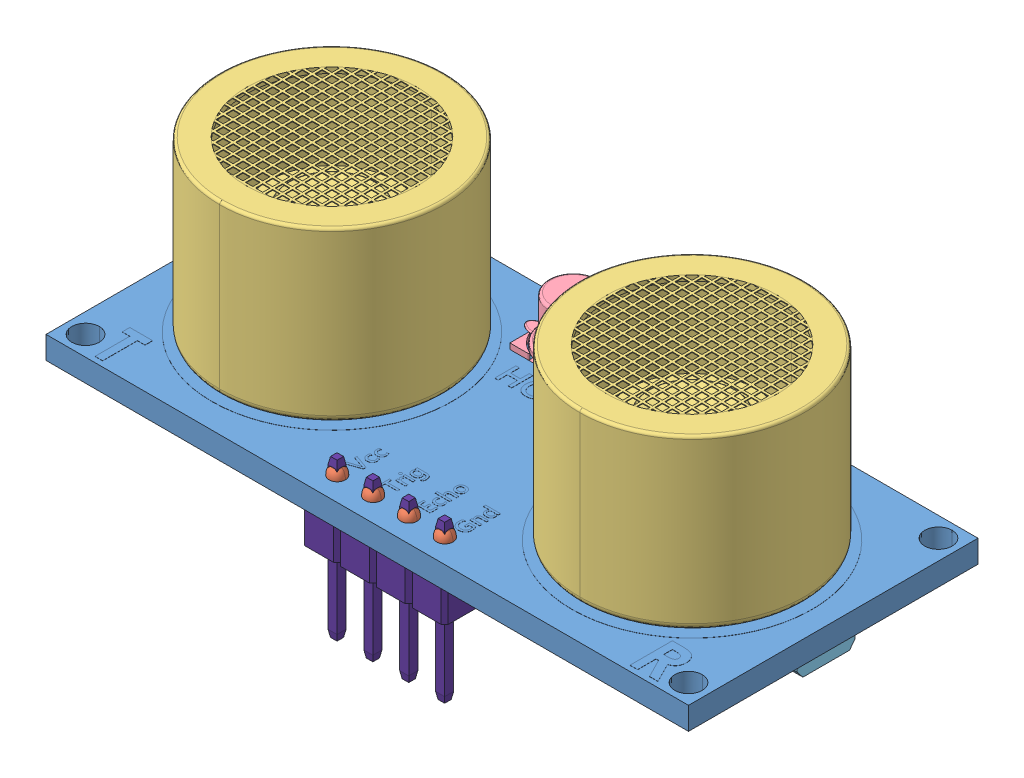
SolidWorks assembly mc_HC-SR04, configuration По умолчанию. Lengths in mm.
Overall size (45.5 21.95 20.5).
46 component instances, 17 part files, 0 mates.
Components (placement in the parent):
- HC-SR04.STEP-1: HC-SR04.STEP [Default] at origin size (45.5 21.95 20.5)
  - HC-SR04board.STEP-1: HC-SR04board.STEP [Default] at origin size (45.5 1.61 20.5)
  - solder.STEP-1: solder.STEP [Default] at (-3.8014 1.6 8.5727) size (1.17 0.65 1.17)
  - solder.STEP-2: solder.STEP [Default] at (-1.2614 1.6 8.5727) size (1.17 0.65 1.17)
  - solder.STEP-3: solder.STEP [Default] at (1.2786 1.6 8.5727) size (1.17 0.65 1.17)
  - solder.STEP-4: solder.STEP [Default] at (3.8186 1.6 8.5727) size (1.17 0.65 1.17)
  - Emitter.STEP-1: Emitter.STEP [Default] at (-12.75 1.6 0) size (15.9 15.2 15.9)
  - Emitter.STEP-2: Emitter.STEP [Default] at (12.75 1.6 0) size (15.9 15.2 15.9)
  - CrystalOscillator.STEP-1: CrystalOscillator.STEP [Default] at (0 1.6 -7.5) size (13.3 6.4 4.5)
  - solder.STEP-5: solder.STEP [Default] at (-2.0167 0 -7.5286) x (-0.837169 0 -0.546944) z (-0.546944 0 0.837169) size (1.17 0.65 1.17)
  - solder.STEP-6: solder.STEP [Default] at (1.9833 0 -7.5286) x (-0.837169 0 -0.546944) z (-0.546944 0 0.837169) size (1.17 0.65 1.17)
  - smdChip14pin.STEP-1: smdChip14pin.STEP [Default] at (22.25 -0.725 0) x (0 0 -1) z (-1 0 0) size (7.3 1.22 8.75)
  - smdChip14pin.STEP-2: smdChip14pin.STEP [Default] at (4.375 -0.725 0) x (0 0 -1) z (-1 0 0) size (7.3 1.22 8.75)
  - smdChip16pin.STEP-1: smdChip16pin.STEP [Default] at (-18.6 -0.725 5) x (1 0 0) z (0 0 -1) size (7.3 1.22 10)
  - smdceramiccapacitor.STEP-1: smdceramiccapacitor.STEP [Default] at (17.8499 0 -5.5522) x (0 0 -1) z (-1 0 0) size (2.52 0.61 1.3)
  - smdceramiccapacitor.STEP-2: smdceramiccapacitor.STEP [Default] at (17.8499 0 5.585) x (0 0 -1) z (-1 0 0) size (2.52 0.61 1.3)
  - smdceramiccapacitor.STEP-3: smdceramiccapacitor.STEP [Default] at (15.2359 0 8.7006) x (-1 0 0) z (0 0 1) size (2.52 0.61 1.3)
  - smdceramiccapacitor.STEP-4: smdceramiccapacitor.STEP [Default] at (8.3844 0 0.0383) x (-1 0 0) z (0 0 1) size (2.52 0.61 1.3)
  - smdceramiccapacitor.STEP-5: smdceramiccapacitor.STEP [Default] at (8.3844 0 -4.7577) x (-1 0 0) z (0 0 1) size (2.52 0.61 1.3)
  - smdceramiccapacitor.STEP-6: smdceramiccapacitor.STEP [Default] at (8.3844 0 -2.3108) x (-1 0 0) z (0 0 1) size (2.52 0.61 1.3)
  - smdceramiccapacitor.STEP-7: smdceramiccapacitor.STEP [Default] at (-7.8145 0 -2.3108) x (-1 0 0) z (0 0 1) size (2.52 0.61 1.3)
  - smdResistor753.STEP-1: smdResistor753.STEP [Default] at (20.6199 0 5.0565) x (-1 0 0) z (0 0 1) size (2.53 0.63 1.31)
  - smdResistor753.STEP-2: smdResistor753.STEP [Default] at (-7.7732 0 -0.1429) x (-1 0 0) z (0 0 1) size (2.53 0.63 1.31)
  - smdResistor753.STEP-3: smdResistor753.STEP [Default] at (20.6199 0 -4.936) x (-1 0 0) z (0 0 1) size (2.53 0.63 1.31)
  - smdResistor392.STEP-1: smdResistor392.STEP [Default] at (-18.578 0 -6.4389) x (-1 0 0) z (0 0 1) size (2.53 0.63 1.31)
  - smdResistor103.STEP-1: smdResistor103.STEP [Default] at (-18.578 0 6.8031) x (-1 0 0) z (0 0 1) size (2.53 0.63 1.31)
  - smdResistor124.STEP-1: smdResistor124.STEP [Default] at (-7.7732 0 1.8639) x (-1 0 0) z (0 0 1) size (2.53 0.63 1.31)
  - smdResistor103.STEP-2: smdResistor103.STEP [Default] at (-7.7732 0 3.8148) x (-1 0 0) z (0 0 1) size (2.53 0.63 1.31)
  - smdResistor103.STEP-3: smdResistor103.STEP [Default] at (-7.7732 0 5.8773) x (-1 0 0) z (0 0 1) size (2.53 0.63 1.31)
  - smdResistor335.STEP-1: smdResistor335.STEP [Default] at (-7.7732 0 -4.435) x (-1 0 0) z (0 0 1) size (2.53 0.63 1.31)
  - smdResistor102.STEP-1: smdResistor102.STEP [Default] at (8.4383 0 5.8773) x (-1 0 0) z (0 0 1) size (2.53 0.63 1.31)
  - smdResistor103.STEP-4: smdResistor103.STEP [Default] at (8.4383 0 3.8148) x (-1 0 0) z (0 0 1) size (2.53 0.63 1.31)
  - smdResistor563.STEP-1: smdResistor563.STEP [Default] at (8.4383 0 1.8639) x (-1 0 0) z (0 0 1) size (2.53 0.63 1.31)
  - smdResistor103.STEP-5: smdResistor103.STEP [Default] at (8.4383 0 -6.6305) x (-1 0 0) z (0 0 1) size (2.53 0.63 1.31)
  - smdResistor622.STEP-1: smdResistor622.STEP [Default] at (9.6708 0 8.6421) x (-1 0 0) z (0 0 1) size (2.53 0.63 1.31)
  - smdResistor124.STEP-2: smdResistor124.STEP [Default] at (10.2038 0 -8.7291) x (-1 0 0) z (0 0 1) size (2.53 0.63 1.31)
  - smdResistor412.STEP-1: smdResistor412.STEP [Default] at (14.0013 0 -8.7291) x (-1 0 0) z (0 0 1) size (2.53 0.63 1.31)
  - smdResistor103.STEP-6: smdResistor103.STEP [Default] at (17.3324 0 -8.7291) x (-1 0 0) z (0 0 1) size (2.53 0.63 1.31)
  - solder.STEP-7: solder.STEP [Default] at (-12.8084 0 -5.0269) x (-0.837169 0 -0.546944) z (-0.546944 0 0.837169) size (1.17 0.65 1.17)
  - solder.STEP-8: solder.STEP [Default] at (-12.8084 0 5.0295) x (-0.837169 0 -0.546944) z (-0.546944 0 0.837169) size (1.17 0.65 1.17)
  - solder.STEP-9: solder.STEP [Default] at (12.7872 0 5.0295) x (-0.837169 0 -0.546944) z (-0.546944 0 0.837169) size (1.17 0.65 1.17)
  - solder.STEP-10: solder.STEP [Default] at (12.7872 0 -5.0269) x (-0.837169 0 -0.546944) z (-0.546944 0 0.837169) size (1.17 0.65 1.17)
  - headerMale.STEP-1: headerMale.STEP [Default] at (3.81 0 8.58) x (-1 0 0) z (0 0 1) size (2.54 11.1 2.54)
  - headerMale.STEP-2: headerMale.STEP [Default] at (1.27 0 8.58) x (-1 0 0) z (0 0 1) size (2.54 11.1 2.54)
  - headerMale.STEP-3: headerMale.STEP [Default] at (-1.27 0 8.58) x (-1 0 0) z (0 0 1) size (2.54 11.1 2.54)
  - headerMale.STEP-4: headerMale.STEP [Default] at (-3.81 0 8.58) x (-1 0 0) z (0 0 1) size (2.54 11.1 2.54)
